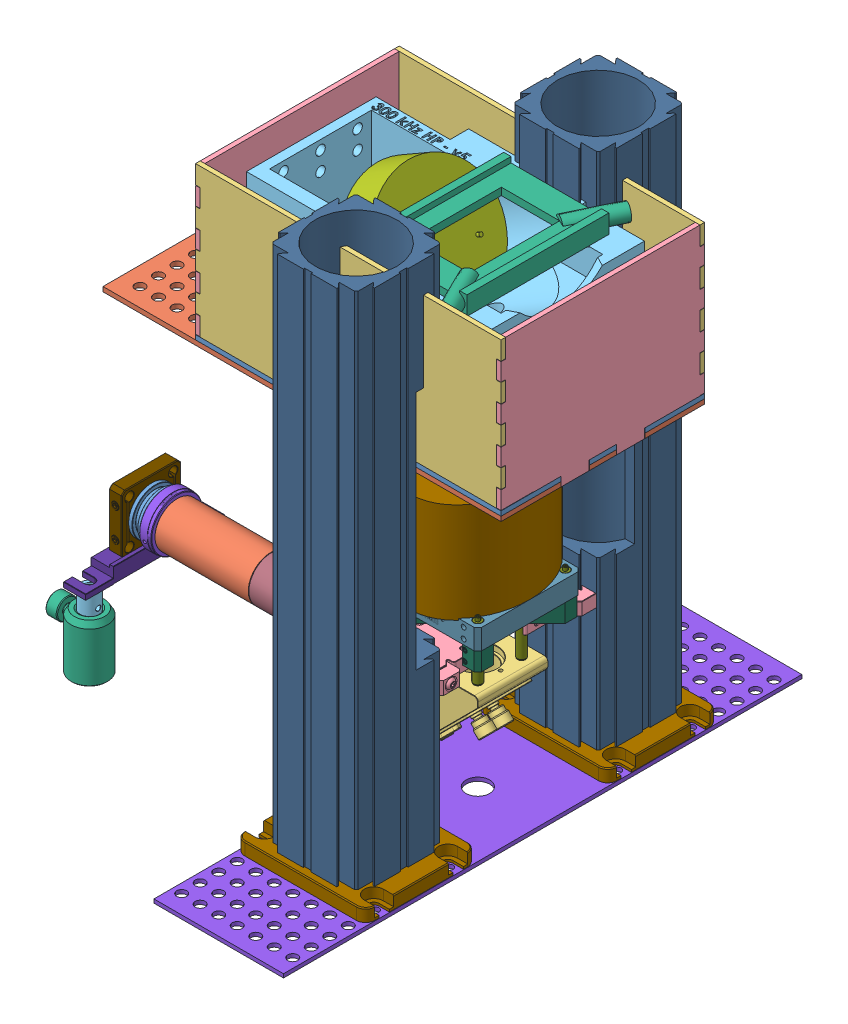
SolidWorks assembly Water Bath, configuration Default. Lengths in mm.
Overall size (337.06 394 355.6).
51 component instances, 28 part files, 28 mates.
Components (placement in the parent):
- WB_0p125_BaseThreaded-1: WB_0p125_BaseThreaded [Default] at (0 3.175 0) size (209.55 3.17 139.7)
- WB_0p125_Base-1: WB_0p125_Base [Default] at origin size (273.05 3.17 139.7)
- WB_0p125_Long-1: WB_0p125_Long [Default] at (0 57.15 -69.85) size (209.55 107.95 3.17)
- WB_0p125_Long-2: WB_0p125_Long [Default] at (0 57.15 66.675) size (209.55 107.95 3.17)
- WB_0p125_Short-1: WB_0p125_Short [Default] at (101.6 57.15 0) x (0 0 1) z (0 1 0) size (139.7 3.17 107.95)
- WB_0p125_Short-2: WB_0p125_Short [Default] at (-104.775 57.15 0) x (0 0 1) z (0 1 0) size (139.7 3.17 107.95)
- 300 kHz Tank HP (5) Opticell-1: 300 kHz Tank HP (5) Opticell [Default] at (19.05 95.25 0) size (171.45 88.9 114.3)
- Opticell-1: Opticell [Default] at (23.9788 95.275 -0.195) size (76.36 12.75 129.72)
- HP Tx-1: HP Tx [Default] at (-29.075 64.925 0) x (0.498711 -0.863793 0.071763) z (-0.035882 0.062149 0.997422) size (83.8 58.17 83.8)
- Table SubAssembly-1: Table SubAssembly [Default] at (-19.05 -237.82 0) x (0 0 -1) z (1 0 0) size (355.6 366.78 89.6)
  - Table-1: Table [Default] at origin size (355.6 2.54 88.9)
  - XT66P1-Solidworks-1: XT66P1-Solidworks [Default] at (-83.0224 2.286 37.592) x (-1 0 0) z (0 0 -1) size (76.2 8.89 89.28)
  - XT66P1-Solidworks-2: XT66P1-Solidworks [Default] at (83.0224 2.286 37.592) size (76.2 8.89 89.28)
  - KCB1-Solidworks-1: KCB1-Solidworks [Default] at (-24.13 99.7796 13.4747) x (0.000001 0 1) z (0 1 0) size (51.13 48.26 51.1) (hidden)
  - RCA1-Solidworks-1: RCA1-Solidworks [Default] at (-24.2926 205.6203 66.0649) x (0 0 -1) z (0 -1 0) size (56.5 73.55 8.89) (hidden)
  - RCA1-Solidworks-2: RCA1-Solidworks [Default] at (24.2926 108.2389 66.0649) x (0 0 -1) z (0 1 0) size (56.5 73.55 8.89) (hidden)
  - XT66-500-modified_v2-1: XT66-500-modified_v2 [Default] at (-83.0224 511.176 37.592) x (0 0 -1) z (0 -1 0) size (66.02 67.06 355.6)
  - XT66-500-modified_v2-2: XT66-500-modified_v2 [Default] at (83.0224 511.176 37.592) x (0 0 1) z (0 -1 0) size (66.02 67.06 355.6)
- Small Condenser Adjustable Sub-Assembly-1: Small Condenser Adjustable Sub-Assembly [Default] at (54.61 -106.3498 20.3199) x (0 -1 0) z (0 0 1) size (256.9 286.9 106.71)
  - LB1437-Solidworks-1: LB1437-Solidworks [Default] at (76.2 -223.413 -20.3199) x (0.879994 0 -0.474985) z (0 -1 0) size (25.4 25.4 3.05)
  - LB1761-Solidworks-1: LB1761-Solidworks [Default] at (76.2 -78.613 -20.3199) x (0.962182 0 -0.272406) z (0 -1 0) size (25.4 25.4 8.98)
  - SM1L40-Solidworks-1: SM1L40-Solidworks [Default] at (78.3398 -122.5422 -22.1696) x (-0.992854 0 -0.119336) z (0 1 0) size (30.48 30.48 105.41)
  - CSA1003-Solidworks-1: CSA1003-Solidworks [Default] at (47.6181 -122.449 -34.035) x (0 -1 0) z (0 0 1) size (71.12 13.97 71.12)
  - LCP02-Solidworks-1: LCP02-Solidworks [Default] at (20.32 -35.5599 -20.32) x (0 0 -1) z (1 0 0) size (70.75 70.61 12.7)
  - ER1-Solidworks-1: ER1-Solidworks [Default] at (36.8841 -51.9737 -4.6825) x (0 -0.925141 -0.379624) z (0 -0.379624 0.925141) size (5.99 30.48 5.99)
  - ER1-Solidworks-3: ER1-Solidworks [Default] at (36.8841 -50.6608 -33.7724) x (0 -0.769482 0.638668) z (0 0.638668 0.769482) size (5.99 30.48 5.99)
  - ER1-Solidworks-4: ER1-Solidworks [Default] at (41.8559 -21.5595 -36.5057) x (0 -0.998351 -0.057413) z (0 0.057413 -0.998351) size (5.99 30.48 5.99)
  - CPB1-Solidworks-2: CPB1-Solidworks [Default] at (105.41 -256.9972 27.3051) x (0 0 1) z (0 -1 0) size (95.25 10.79 15.24)
  - CP08-Solidworks-2: CP08-Solidworks [Default] at (76.2 -263.9822 -20.3199) x (0 0 -1) z (0 1 0) size (41.5 40.64 8.89)
  - SM1T2-Solidworks-1: SM1T2-Solidworks [Default] at (76.2 -248.6152 -20.3199) x (0.998592 0 -0.053039) z (0 1 0) size (31.75 31.75 12.7)
  - SM1L25-Solidworks-1: SM1L25-Solidworks [Default] at (139.9124 -186.275 -15.6668) x (0 -1 0) z (-0.806632 0 -0.591053) size (67.31 30.48 30.48)
  - CPB1-Solidworks-3: CPB1-Solidworks [Default] at (105.41 -62.23 27.3051) x (0 0 1) z (0 -1 0) size (95.25 10.79 15.24)
  - CP08-Solidworks-3: CP08-Solidworks [Default] at (76.2 -69.215 -20.3199) x (0 0 -1) z (0 1 0) size (41.5 40.64 8.89)
  - KCB1-Solidworks-2: KCB1-Solidworks [Default] at (100.33 -11.43 3.8101) x (-1 0 0) z (0 -1 0) size (51.13 48.26 51.1)
  - ER1-Solidworks-6: ER1-Solidworks [Default] at (36.8841 -20.7263 -3.7781) x (0 -0.795862 0.605478) z (0 0.605478 0.795862) size (5.99 30.48 5.99)
  - RCA2-Solidworks-1: RCA2-Solidworks [Default] at (68.2294 -49.0321 -29.2771) x (0 1 0) z (-1 0 0) size (56.73 41.06 8.89)
  - RCA2-Solidworks-2: RCA2-Solidworks [Default] at (68.2294 -22.0879 -11.3628) x (0 -1 0) z (-1 0 0) size (56.73 41.06 8.89)
  - TR075-Solidworks-1: TR075-Solidworks [Default] at (105.41 -263.9822 17.7801) x (0 0 -1) z (0 -1 0) size (12.67 19.05 12.87)
  - TR075-Solidworks-2: TR075-Solidworks [Default] at (143.51 -263.9822 17.7801) x (0 0 1) z (0 -1 0) size (12.67 19.05 12.87)
  - PH1.5-Solidworks-1: PH1.5-Solidworks [Default] at (136.906 -263.9822 17.7801) x (0 0 1) z (0 -1 0) size (25 38.71 35.41)
  - ER05-Solidworks-1: ER05-Solidworks [Default] at (92.6015 -68.5259 -5.9839) x (0.310188 0 -0.950675) z (0.950675 0 0.310188) size (5.99 17.78 5.99)
  - ER05-Solidworks-2: ER05-Solidworks [Default] at (59.8613 -68.5259 -4.5371) x (-0.22668 0 0.973969) z (-0.973969 0 -0.22668) size (5.99 17.78 5.99)
  - ER05-Solidworks-3: ER05-Solidworks [Default] at (92.2659 -68.5259 -34.1935) size (5.99 17.78 5.99)
  - ER05-Solidworks-4: ER05-Solidworks [Default] at (59.7556 -68.5259 -34.7555) x (-0.375833 0 0.926687) z (-0.926687 0 -0.375833) size (5.99 17.78 5.99)
  - SM1D12D-Solidworks-1: SM1D12D-Solidworks [Default] at (81.3975 -244.783 -22.8892) x (0.973299 0 -0.22954) z (0 1 0) size (35.81 35.81 11.94)
  - SM1D12D-Solidworks-2: SM1D12D-Solidworks [Default] at (70.9424 -73.1298 -22.7639) x (-0.788375 0 -0.615195) z (0 1 0) size (35.81 35.81 11.94)
  - ER1-Solidworks-9: ER1-Solidworks [Default] at (15.1859 -4.2179 -49.5429) x (0 0.95877 -0.284182) z (0 0.284182 0.95877) size (5.99 30.48 5.99)
  - ER1-Solidworks-10: ER1-Solidworks [Default] at (15.1859 -64.6339 -49.076) x (0 0.993069 0.117534) z (0 -0.117534 0.993069) size (5.99 30.48 5.99)
  - ER1-Solidworks-11: ER1-Solidworks [Default] at (15.1859 -4.6008 10.8986) x (0 0.995869 0.090807) z (0 -0.090807 0.995869) size (5.99 30.48 5.99)
  - ER1-Solidworks-12: ER1-Solidworks [Default] at (15.1859 -64.2349 10.4858) x (0 0.96466 -0.263499) z (0 0.263499 0.96466) size (5.99 30.48 5.99)
  - OlympusCondenser-1: OlympusCondenser [Default] at (7.0104 -35.56 -20.3199) x (0 -1 0) z (0 0 -1) size (71.12 107.95 91.44)
Mates (geometry in assembly coordinates):
- Coincident1: coincident aligned: plane of WB_0p125_BaseThreaded-1 through (-101.6 6.35 66.675) normal (0 0 1); plane of WB_0p125_Base-1 through (-101.6 3.175 66.675) normal (0 0 1)
- Coincident2: coincident aligned: plane of WB_0p125_BaseThreaded-1 through (101.6 6.35 66.675) normal (1 0 0); plane of WB_0p125_Base-1 through (101.6 3.175 66.675) normal (1 0 0)
- Coincident3: coincident anti-aligned: plane of WB_0p125_BaseThreaded-1 through (0 3.175 0) normal (0 -1 0); plane of WB_0p125_Base-1 through (0 3.175 0) normal (0 1 0)
- Coincident4: coordinate: point of WB_0p125_Base-1; point of assembly
- Coincident5: coincident aligned: plane of WB_0p125_BaseThreaded-1 through (101.6 6.35 66.675) normal (1 0 0); plane of WB_0p125_Long-2 through (101.6 6.35 69.85) normal (1 0 0)
- Coincident6: coincident anti-aligned: plane of WB_0p125_BaseThreaded-1 through (0 6.35 0) normal (0 1 0); plane of WB_0p125_Long-2 through (-101.6 6.35 69.85) normal (0 -1 0)
- Coincident8: coincident anti-aligned: plane of WB_0p125_BaseThreaded-1 through (0 6.35 0) normal (0 1 0); plane of WB_0p125_Long-1 through (-101.6 6.35 -66.675) normal (0 -1 0)
- Coincident9: coincident aligned: plane of WB_0p125_BaseThreaded-1 through (-101.6 6.35 66.675) normal (-1 0 0); plane of WB_0p125_Long-1 through (-101.6 6.35 -66.675) normal (-1 0 0)
- Coincident11: coincident anti-aligned: plane of WB_0p125_BaseThreaded-1 through (-101.6 6.35 66.675) normal (-1 0 0); plane of WB_0p125_Short-2 through (-101.6 57.15 0) normal (1 0 0)
- Coincident12: coincident anti-aligned: plane of WB_0p125_BaseThreaded-1 through (0 6.35 0) normal (0 1 0); plane of WB_0p125_Short-2 through (-101.6 6.35 -66.675) normal (0 -1 0)
- Coincident14: coincident anti-aligned: plane of WB_0p125_Long-2 through (0 57.15 66.675) normal (0 0 -1); plane of WB_0p125_Short-2 through (-101.6 107.95 66.675) normal (0 0 1)
- Coincident16: coincident anti-aligned: plane of WB_0p125_Long-2 through (0 57.15 66.675) normal (0 0 -1); plane of WB_0p125_Short-1 through (104.775 107.95 66.675) normal (0 0 1)
- Coincident18: coincident anti-aligned: plane of WB_0p125_Long-1 through (0 57.15 -66.675) normal (0 0 1); plane of WB_0p125_Short-2 through (-101.6 107.95 -66.675) normal (0 0 -1)
- Coincident19: coincident anti-aligned: plane of WB_0p125_BaseThreaded-1 through (-101.6 6.35 -66.675) normal (0 0 -1); plane of WB_0p125_Long-1 through (0 57.15 -66.675) normal (0 0 1)
- Coincident20: coincident aligned: plane of WB_0p125_Long-2 through (104.775 107.95 66.675) normal (1 0 0); plane of WB_0p125_Short-1 through (104.775 57.15 0) normal (1 0 0)
- Coincident21: coincident aligned: plane of WB_0p125_Base-1 through (0 0 0) normal (0 -1 0); plane of WB_0p125_Short-1 through (104.775 0 9.525) normal (0 -1 0)
- Concentric3: concentric aligned: circle of WB_0p125_BaseThreaded-1; circle of 300 kHz Tank HP (5) Opticell-1
- Concentric4: concentric aligned: circle of WB_0p125_BaseThreaded-1; circle of 300 kHz Tank HP (5) Opticell-1
- Coincident23: coincident anti-aligned: plane of WB_0p125_BaseThreaded-1 through (0 6.35 0) normal (0 1 0); plane of 300 kHz Tank HP (5) Opticell-1 through (19.05 6.35 0) normal (0 -1 0)
- Coincident24: coincident anti-aligned: plane of 300 kHz Tank HP (5) Opticell-1 through (19.05 88.9 0) normal (0 1 0); plane of Opticell-1 through (23.9788 88.9 -0.195) normal (0 -1 0)
- Coincident25: coincident anti-aligned: plane of 300 kHz Tank HP (5) Opticell-1 through (-12.0762 88.9 -48.895) normal (1 0 0); plane of Opticell-1 through (-12.0762 97.775 48.505) normal (-1 0 0)
- Coincident26: coincident anti-aligned: plane of 300 kHz Tank HP (5) Opticell-1 through (-12.0762 88.9 -48.895) normal (0 0 1); plane of Opticell-1 through (-12.0762 97.775 -48.895) normal (0 0 -1)
- Concentric5: concentric aligned: cylinder of 300 kHz Tank HP (5) Opticell-1 through (-29.075 64.925 0) axis (-0.866025 -0.5 0) radius 42.545; cylinder of HP Tx-1 through (-29.075 64.925 0) axis (-0.866025 -0.5 0) radius 41.9
- Coincident27: coincident anti-aligned: plane of 300 kHz Tank HP (5) Opticell-1 through (-31.0925 68.4194 0) normal (0.866025 0.5 0); plane of HP Tx-1 through (-29.075 64.925 0) normal (-0.866025 -0.5 0)
- Coincident28: coincident anti-aligned: plane of Table SubAssembly-1/Table-1 through (-19.05 -237.82 0) normal (0 0 -1); plane of assembly through (0 0 0) normal (0 0 1)
- Concentric6: concentric aligned: circle of 300 kHz Tank HP (5) Opticell-1; circle of Table SubAssembly-1/Table-1
- Concentric7: concentric aligned: circle of Table SubAssembly-1/Table-1; circle of Small Condenser Adjustable Sub-Assembly-1/OlympusCondenser-1
- Parallel1: parallel aligned: plane of Table SubAssembly-1/XT66-500-modified_v2-1 through (-1.796 -226.644 116.5515) normal (0 0 1); plane of Small Condenser Adjustable Sub-Assembly-1/CSA1003-Solidworks-1 through (54.61 -106.3498 35.56) normal (0 0 1)
